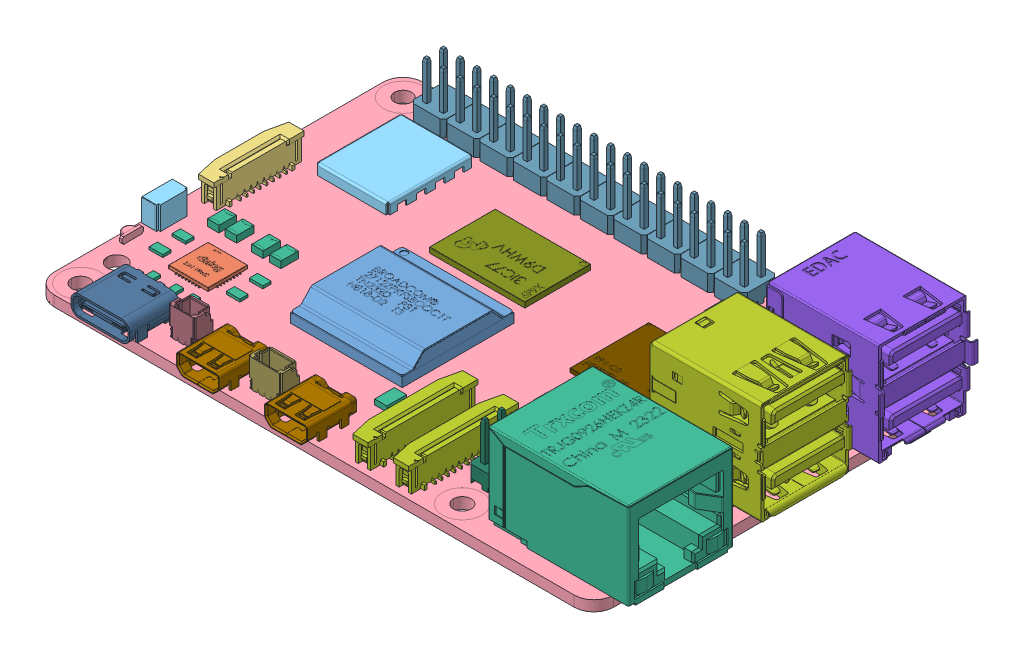
SolidWorks assembly RASPBERRY_PI_5, configuration Default. Lengths in mm.
Overall size (89.04 20.84 57.19).
29 component instances, 25 part files, 0 mates.
Components (placement in the parent):
- RASPBERRY_PI_5.STEP-1: RASPBERRY_PI_5.STEP [Default] at origin size (89.04 20.84 57.19)
  - SLOT_CARD_ASM.STEP-1: SLOT_CARD_ASM.STEP [Default] at (-44.5448 -12.71 -6.4393) x (0 0 -1) z (0 1 0) size (11.95 11.4 1.48)
    - CARD_SLOT_METAL_PIN.STEP-1: CARD_SLOT_METAL_PIN.STEP [Default] at (-3.5293 -7.6678 12.2938) x (0 -1 0) z (1 0 0) size (7.95 0.89 8.04)
    - SD_CARD_V1.STEP-1: SD_CARD_V1.STEP [Default] at (-18.1743 -9.7848 12.71) x (-1 0 0) z (0 0 -1) size (11.71 10.28 1.3)
    - PART3_V1.STEP-1: PART3_V1.STEP [Default] at (-6.4643 -9.3448 11.38) x (1 0 0) z (0 0 -1) size (11.95 11.4 1.45)
  - PLATE_RASPBERRY_PI_5.STEP-1: PLATE_RASPBERRY_PI_5.STEP [Default] x (1 0 0) z (0 1 0) size (85 56 1.7)
  - METAL_PLATE..STEP-1: METAL_PLATE..STEP [Default] at (-30 3 -14.2) x (1 0 0) z (0 1 0) size (11.01 13.01 1.6)
  - GIGABIT_ETHERNET_PORT.STEP-1: GIGABIT_ETHERNET_PORT.STEP [Default] at (45.5 8.525 17.8) x (0 0 -1) z (1 0 0) size (16.1 17.2 21.45)
  - 2xUSB_3.0_PORT.STEP-1: 2xUSB_3.0_PORT.STEP [Default] at (28.53 10.58 -1.1) x (0 1 0) z (1 0 0) size (20.65 15.33 17.66)
  - 2xUSB_2.0_PORT.STEP-1: 2xUSB_2.0_PORT.STEP [Default] at (28.53 9.4 -19) x (0 1 0) z (1 0 0) size (19.16 15.33 17.86)
  - FEMALE_MICRO_HDMI_CONNECTOR.STEP-1: FEMALE_MICRO_HDMI_CONNECTOR.STEP [Default] at (-16.7 3.05 21.5) size (6.5 3.51 7.5)
  - FEMALE_MICRO_HDMI_CONNECTOR.STEP-2: FEMALE_MICRO_HDMI_CONNECTOR.STEP [Default] at (-3.3 3.05 21.5) size (6.5 3.51 7.5)
  - FEMALE_USB_CONNECTOR.STEP-1: FEMALE_USB_CONNECTOR.STEP [Default] at (-31.3 3.18 21.58) size (8.94 3.96 7.9)
  - STOCK_1.STEP-1: STOCK_1.STEP [Default] at (0.2694 -0.16 -24.2409) x (1 0 0) z (0 1 0) size (3.61 6 4.35)
  - STOCK_2.STEP-1: STOCK_2.STEP [Default] at (-10.7909 -0.16 48.1306) x (0 0 -1) z (0 1 0) size (3.61 5 4.35)
  - STOCK_3.STEP-1: STOCK_3.STEP [Default] at (-24.6409 -0.16 47.3806) x (0 0 -1) z (0 1 0) size (3.61 4 4.35)
  - 3.0_PIN_HEADER_10.STEP-1: 3.0_PIN_HEADER_10.STEP [Default] at (-32.86 4.1 -24.5) x (0 0 -1) z (0 1 0) size (5.08 50.8 11.8)
  - 2.0_PIN_HEADER.STEP-1: 2.0_PIN_HEADER.STEP [Default] at (19.04 4.1 18.56) x (1 0 0) z (0 1 0) size (5.08 5.08 11.8)
  - 9FD77_D9WHV.STEP-1: 9FD77_D9WHV.STEP [Default] at (-9.25 1.6 -11) x (0 0 1) z (0 1 0) size (10 14.5 0.8)
  - GIGABIT_ETHERNET_TRANSCEIVER.STEP-1: GIGABIT_ETHERNET_TRANSCEIVER.STEP [Default] at (21.5315 1.6 4.5573) x (0.707107 0 0.707107) z (0 1 0) size (6.9 6.9 1.1)
  - RP1_CO_CONTROLLER.STEP-1: RP1_CO_CONTROLLER.STEP [Default] at (15.9 1.6 -6.95) x (0 0 1) z (0 1 0) size (12 12 0.7)
  - BROADCOM_1.STEP-1: BROADCOM_1.STEP [Default] at (-0.825 4.78 5.305) x (0 0 1) z (-1 0 0) size (17 3.38 17)
  - MxL.STEP-1: MxL.STEP [Default] at (-31.24 1.6 12.88) x (0 0 1) z (0 1 0) size (6.48 6.48 0.6)
  - CAMERA_DISPLAY_1.STEP-1: CAMERA_DISPLAY_1.STEP [Default] at (-45.8516 -0.0005 -20.0821) x (1 0 0) z (0 1 0) size (3.5 13.7 3.9)
  - BUTTON_MINI.STEP-1: BUTTON_MINI.STEP [Default] at (0.19 4.2 29.7) x (1 0 0) z (0 -1 0) size (1.45 3.2 1)
  - BUTTON_2.STEP-1: BUTTON_2.STEP [Default] at (-41 1.6 9.6006) x (0 0 1) z (0 1 0) size (4.65 2.9 3.5)
  - CONNECT_V1.STEP-1: CONNECT_V1.STEP [Default] at (-5.5164 1.6 -0.8649) x (1 0 0) z (0 1 0) size (65.38 41.11 2)
  - CAMERA_DISPLAY_2.STEP-1: CAMERA_DISPLAY_2.STEP [Default] at (0.0484 -0.0005 -0.5921) x (1 0 0) z (0 1 0) size (3.5 16.7 3.9)
  - CAMERA_DISPLAY_2.STEP-2: CAMERA_DISPLAY_2.STEP [Default] at (6.2484 -0.0005 -0.5921) x (1 0 0) z (0 1 0) size (3.5 16.7 3.9)
